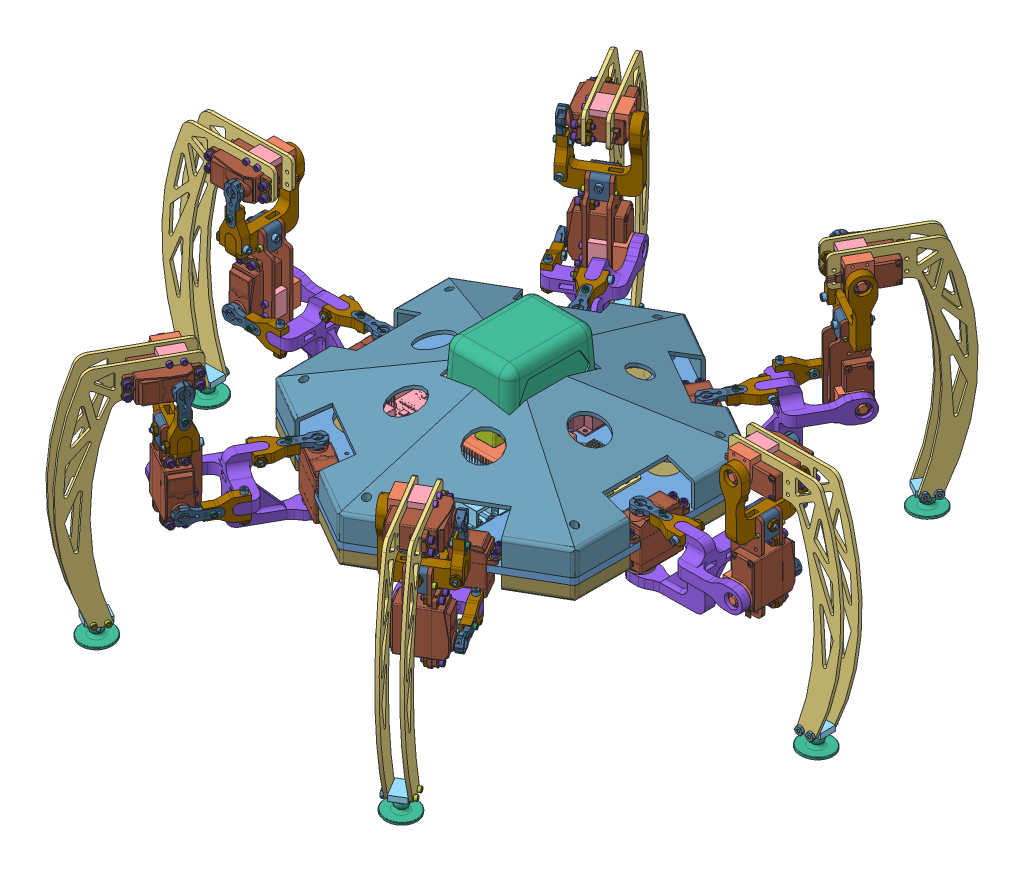
SolidWorks assembly Hexapod_(Hexagonal), configuration Défaut. Lengths in mm.
Overall size (628.94 223.3 579.2).
540 component instances, 32 part files, 38 mates.
Components (placement in the parent):
- Body_(Hexagonal)-1: Body_(Hexagonal) [Défaut] at origin size (278.74 6 320)
- Battery_holder-1: Battery_holder [Default] at (0 14.35 0) x (0 0 1) z (-1 0 0) size (60 19.6 60)
- 12Channel PWM-1: 12Channel PWM [Default] at (77.5 3 0) size (25.4 7.55 66.7)
- 12Channel PWM-2: 12Channel PWM [Default] at (47.4 3 0) size (25.4 7.55 66.7)
- arduinoMega-2: arduinoMega [Detailed] at (-61.35 5 1.27) x (0 0 -1) z (1 0 0) size (108.32 14.5 53.3)
- raspberryPi3B-1: raspberryPi3B [Detailed] at (12.5 5.5 63.95) x (1 0 0) z (0 1 0) size (87.05 58.5 19.5)
- Battery-1: Battery [Défaut] at (0.5853 59.4876 -93.4347) x (-1 0 0) z (0 0 1) size (64.47 74.3 85.78)
  - MAKITA 4.0AH-1: MAKITA 4.0AH [Défaut] at (0.5853 -29.7874 85.4436) size (64.47 57.15 85.78)
  - MAKITA 4.0AH MOBILE-1: MAKITA 4.0AH MOBILE [Défaut] at (0.5853 -39.3124 91.7936) size (45.84 26.68 66.29)
- Foot+Tibia+Femur-1: Foot+Tibia+Femur [Défaut] at (-119.0679 -25 20.1) size (210.19 223.27 63.83) (flexible)
  - Femur-1: Femur [Défaut] at origin size (137.43 61.64 61.08) (flexible)
    - Joint_(Femur_to_tibia)-1: Joint_(Femur_to_tibia) [Défaut] at (-66.4348 29.5 -48.8085) x (0.999924 0 -0.012321) z (0.012321 0 0.999924) size (122 58.8 58.8)
    - Horn_attachment-3: Horn_attachment [Défaut] at (-38.1979 44.8 -29.755) x (0.999924 0 -0.012321) z (0 1 0) size (33 20 8)
    - Horn-3: Horn [Défaut] at (-10.2 48.8 -30.1) x (-0.999924 0 0.012321) z (0 1 0) size (35.39 15.87 6)
    - DS3225MG-3: DS3225MG [Default] at (-10.2 45.8 -30.1) x (0 0 1) z (0 1 0) size (57.25 20.4 45.91)
    - Bearing_mount_(Femur)-1: Bearing_mount_(Femur) [Default] at (2.5 22 -30.1) x (1 0 0) z (0 -1 0) size (35.3 20.2 31)
    - Bearing-3: Bearing [Default] at (-10.2 -6.7498 -30.1) x (0.400474 0 0.916308) z (-0.916308 0 0.400474) size (13.87 4.75 13.87)
    - MSHXNUT 0.112-40-D-N-1: MSHXNUT 0.112-40-D-N [MSHXNUT 0.112-40-D-N] at (-30.1985 40.8 -29.8536) x (-0.510633 0 -0.859799) z (0 1 0) size (6.35 7.33 2.49)
    - HX-SHCS 0.112-40x0.4375x0.4375-N-1: HX-SHCS 0.112-40x0.4375x0.4375-N [HX-SHCS 0.112-40x0.4375x0.4375-N] at (-30.1985 51.6448 -29.8536) x (0 -1 0) z (-0.489292 0 0.87212) size (13.96 4.65 4.65)
    - Narrow FW 0.138-1: Narrow FW 0.138 [Narrow FW 0.138] at (-15.2 31.2 4.7) x (0 -1 0) z (-0.829316 0 -0.55878) size (0.81 7.92 7.92)
    - HX-SHCS 0.138-32x0.5x0.5-N-1: HX-SHCS 0.138-32x0.5x0.5-N [HX-SHCS 0.138-32x0.5x0.5-N] at (-15.2 35.772 4.7) x (0 -1 0) z (0.866025 0 -0.5) size (16.21 5.74 5.74)
    - Narrow FW 0.138-2: Narrow FW 0.138 [Narrow FW 0.138] at (-15.2 31.2 -44.9) x (0 -1 0) z (-0.829316 0 -0.55878) size (0.81 7.92 7.92)
    - Narrow FW 0.138-3: Narrow FW 0.138 [Narrow FW 0.138] at (-5.2 31.2 4.7) x (0 -1 0) z (-0.829316 0 -0.55878) size (0.81 7.92 7.92)
    - Narrow FW 0.138-4: Narrow FW 0.138 [Narrow FW 0.138] at (-5.2 31.2 -44.9) x (0 -1 0) z (-0.829316 0 -0.55878) size (0.81 7.92 7.92)
    - HX-SHCS 0.138-32x0.5x0.5-N-2: HX-SHCS 0.138-32x0.5x0.5-N [HX-SHCS 0.138-32x0.5x0.5-N] at (-15.2 35.772 -44.9) x (0 -1 0) z (0.866025 0 -0.5) size (16.21 5.74 5.74)
    - HX-SHCS 0.138-32x0.5x0.5-N-3: HX-SHCS 0.138-32x0.5x0.5-N [HX-SHCS 0.138-32x0.5x0.5-N] at (-5.2 35.772 4.7) x (0 -1 0) z (0.866025 0 -0.5) size (16.21 5.74 5.74)
    - HX-SHCS 0.138-32x0.5x0.5-N-4: HX-SHCS 0.138-32x0.5x0.5-N [HX-SHCS 0.138-32x0.5x0.5-N] at (-5.2 35.772 -44.9) x (0 -1 0) z (0.866025 0 -0.5) size (16.21 5.74 5.74)
    - MSHXNUT 0.138-32-D-N-1: MSHXNUT 0.138-32-D-N [MSHXNUT 0.138-32-D-N] at (-52.0379 44.8 -16.6879) x (-0.86596 -0.5 0.010671) z (0.012321 0 0.999924) size (7.92 9.15 2.9)
    - HX-SHCS 0.138-32x1x1-N-2: HX-SHCS 0.138-32x1x1-N [HX-SHCS 0.138-32x1x1-N] at (-52.3632 44.8 -43.0867) x (0.012321 0 0.999924) z (-0.86596 -0.5 0.010671) size (28.91 5.74 5.74)
  - Foot_(Long)-4: Foot_(Long) [Défaut] at (-141.7664 117.7478 -37.8795) x (0.999923 0.001668 -0.012321) z (0.012321 0 0.999924) size (104.1 223.13 60.64) (flexible)
    - DS3225MG-1: DS3225MG [Default] at (30.1 10.2 45.8) x (-1 0 0) z (0 0 1) size (57.25 20.4 45.91)
    - Bearing-1: Bearing [Default] at (30.1 10.2 -6.7498) x (-0.568255 0.822853 0) z (0.822853 0.568255 0) size (13.87 4.75 13.87)
    - Bearing_mount_(Foot)-1: Bearing_mount_(Foot) [Default] at (30.1 22.9 8.1) x (0 1 0) z (0 0 -1) size (25.3 20.2 17.1)
    - Foot_(Long)-1: Foot_(Long) [Default] at (18.7 14 25) size (103.08 208 3)
    - Link-1: Link [Default] at (30.1 22.9 11.1) x (0 -1 0) z (0 0 1) size (5 20.2 13.9)
    - Foot_(Long)-2: Foot_(Long) [Default] at (18.7 14 8.1) size (103.08 208 3)
    - Joint_(Foot_to_slipper)-2: Joint_(Foot_to_slipper) [Default] at (-21.9427 -177.5 11.1) x (0 1 0) z (0 0 1) size (15 20.2 13.9)
    - Horn-1: Horn [Défaut] at (30.1 10.2 48.8) x (-0.007987 -0.999968 0) z (0 0 1) size (35.39 15.87 6)
    - Horn_attachment-1: Horn_attachment [Défaut] at (29.8764 -17.7991 44.8) x (0.007987 0.999968 0) z (0 0 1) size (33 20 8)
    - Slipper-1: Slipper [Défaut] at (-21.7184 -191.9896 17.7406) x (0.999392 0.031392 0.015197) z (-0.013787 -0.044657 0.998907) size (30 10.55 30)
    - HX-SHCS 0.112-40x0.4375x0.4375-N-15: HX-SHCS 0.112-40x0.4375x0.4375-N [HX-SHCS 0.112-40x0.4375x0.4375-N] at (29.9403 -9.7994 51.6448) x (0 0 -1) z (0.869991 0.493067 0) size (13.96 4.65 4.65)
    - MSHXNUT 0.112-40-D-N-7: MSHXNUT 0.112-40-D-N [MSHXNUT 0.112-40-D-N] at (29.9403 -9.7994 40.8) x (-0.007987 -0.999968 0) z (0 0 1) size (6.35 7.33 2.49)
    - HX-SHCS 0.112-40x0.875x0.875-N-9: HX-SHCS 0.112-40x0.875x0.875-N [HX-SHCS 0.112-40x0.875x0.875-N] at (-26.9427 -177.5 30.8448) x (0 0 -1) z (0 1 0) size (25.07 4.65 4.65)
    - MSHXNUT 0.112-40-D-N-4: MSHXNUT 0.112-40-D-N [MSHXNUT 0.112-40-D-N] at (-26.9427 -177.5 8.1) x (0.866025 -0.5 0) z (0 0 1) size (6.35 7.33 2.49)
    - HX-SHCS 0.112-40x0.875x0.875-N-11: HX-SHCS 0.112-40x0.875x0.875-N [HX-SHCS 0.112-40x0.875x0.875-N] at (-16.9427 -177.5 30.8448) x (0 0 -1) z (0 1 0) size (25.07 4.65 4.65)
    - MSHXNUT 0.112-40-D-N-6: MSHXNUT 0.112-40-D-N [MSHXNUT 0.112-40-D-N] at (-16.9427 -177.5 8.1) x (0.866025 -0.5 0) z (0 0 1) size (6.35 7.33 2.49)
    - HX-SHCS 0.112-40x1x0.75-N-13: HX-SHCS 0.112-40x1x0.75-N [HX-SHCS 0.112-40x1x0.75-N] at (25.1 22.9 30.8448) x (0 0 -1) z (0 1 0) size (28.24 4.65 4.65)
    - HX-SHCS 0.112-40x1x0.75-N-14: HX-SHCS 0.112-40x1x0.75-N [HX-SHCS 0.112-40x1x0.75-N] at (35.1 22.9 30.8448) x (0 0 -1) z (0 1 0) size (28.24 4.65 4.65)
    - HX-SHCS 0.138-32x0.5x0.5-N-14: HX-SHCS 0.138-32x0.5x0.5-N [HX-SHCS 0.138-32x0.5x0.5-N] at (-4.7 5.2 35.772) x (0 0 -1) z (0.866025 0.5 0) size (16.21 5.74 5.74)
    - Narrow FW 0.138-1: Narrow FW 0.138 [Narrow FW 0.138] at (-4.7 5.2 31.2) x (0 0 -1) z (-0.829316 0.55878 0) size (0.81 7.92 7.92)
    - MSHXNUT 0.138-32-D-N-1: MSHXNUT 0.138-32-D-N [MSHXNUT 0.138-32-D-N] at (-4.7 5.2 25) x (0.866025 0.5 0) z (0 0 1) size (7.92 9.15 2.9)
    - MSHXNUT 0.138-32-D-N-2: MSHXNUT 0.138-32-D-N [MSHXNUT 0.138-32-D-N] at (44.9 5.2 25) x (0.866025 0.5 0) z (0 0 1) size (7.92 9.15 2.9)
    - MSHXNUT 0.138-32-D-N-3: MSHXNUT 0.138-32-D-N [MSHXNUT 0.138-32-D-N] at (-4.7 15.2 25) x (0.866025 0.5 0) z (0 0 1) size (7.92 9.15 2.9)
    - MSHXNUT 0.138-32-D-N-4: MSHXNUT 0.138-32-D-N [MSHXNUT 0.138-32-D-N] at (44.9 15.2 25) x (0.866025 0.5 0) z (0 0 1) size (7.92 9.15 2.9)
    - HX-SHCS 0.138-32x0.5x0.5-N-15: HX-SHCS 0.138-32x0.5x0.5-N [HX-SHCS 0.138-32x0.5x0.5-N] at (44.9 5.2 35.772) x (0 0 -1) z (0.866025 0.5 0) size (16.21 5.74 5.74)
    - HX-SHCS 0.138-32x0.5x0.5-N-16: HX-SHCS 0.138-32x0.5x0.5-N [HX-SHCS 0.138-32x0.5x0.5-N] at (-4.7 15.2 35.772) x (0 0 -1) z (0.866025 0.5 0) size (16.21 5.74 5.74)
    - HX-SHCS 0.138-32x0.5x0.5-N-17: HX-SHCS 0.138-32x0.5x0.5-N [HX-SHCS 0.138-32x0.5x0.5-N] at (44.9 15.2 35.772) x (0 0 -1) z (0.866025 0.5 0) size (16.21 5.74 5.74)
    - Narrow FW 0.138-2: Narrow FW 0.138 [Narrow FW 0.138] at (44.9 5.2 31.2) x (0 0 -1) z (-0.829316 0.55878 0) size (0.81 7.92 7.92)
    - Narrow FW 0.138-3: Narrow FW 0.138 [Narrow FW 0.138] at (-4.7 15.2 31.2) x (0 0 -1) z (-0.829316 0.55878 0) size (0.81 7.92 7.92)
    - Narrow FW 0.138-4: Narrow FW 0.138 [Narrow FW 0.138] at (44.9 15.2 31.2) x (0 0 -1) z (-0.829316 0.55878 0) size (0.81 7.92 7.92)
  - Tibia-3: Tibia [Défaut] at (-122.5709 19.4647 -38.1161) x (-0.006318 -0.99998 0.000078) z (0.012321 0 0.999924) size (129.02 61.26 61.64) (flexible)
    - Joint_(Tibia_to_foot)-1: Joint_(Tibia_to_foot) [Défaut] at (-62.6 10.2 -10) size (64 20 58.8)
    - DS3225MG-2: DS3225MG [Default] at (-10.1 10.2 45.8) x (-1 0 0) z (0 0 1) size (57.25 20.4 45.91)
    - Link-3: Link [Default] at (-10.1 22.9 11.1) x (0 -1 0) z (0 0 1) size (5 20.2 13.9)
    - Horn-2: Horn [Défaut] at (-10.1 10.2 48.8) x (-0.006319 0.99998 0) z (0 0 1) size (35.39 15.87 6)
    - Horn_attachment-2: Horn_attachment [Défaut] at (-10.2769 38.1994 44.8) x (0.006319 -0.99998 0) z (0 0 1) size (33 20 8)
    - Joint_attachment_(Tibia)-1: Joint_attachment_(Tibia) [Défaut] at (-62.6 10.2 25) size (19 20.4 13.9)
    - Tibia-1: Tibia [Défaut] at (-62.6 10.2 28) size (80 28 3)
    - Tibia-2: Tibia [Défaut] at (-62.6 10.2 11.1) size (80 28 3)
    - Bearing_mount_(Foot)-2: Bearing_mount_(Foot) [Default] at (-10.1 22.9 8.1) x (0 1 0) z (0 0 -1) size (25.3 20.2 17.1)
    - Bearing-2: Bearing [Default] at (-10.1 10.2 -6.7498) x (-0.993915 0.110147 0) z (0.110147 0.993915 0) size (13.87 4.75 13.87)
    - HX-SHCS 0.112-40x0.4375x0.4375-N-1: HX-SHCS 0.112-40x0.4375x0.4375-N [HX-SHCS 0.112-40x0.4375x0.4375-N] at (-10.2264 30.1996 51.6448) x (0 0 -1) z (-0.862849 -0.505462 0) size (13.96 4.65 4.65)
    - MSHXNUT 0.112-40-D-N-1: MSHXNUT 0.112-40-D-N [MSHXNUT 0.112-40-D-N] at (-10.2264 30.1996 40.8) x (-0.006319 0.99998 0) z (0 0 1) size (6.35 7.33 2.49)
    - HX-SHCS 0.112-40x1x0.75-N-1: HX-SHCS 0.112-40x1x0.75-N [HX-SHCS 0.112-40x1x0.75-N] at (-15.1 22.9 30.8448) x (0 0 -1) z (0 1 0) size (28.24 4.65 4.65)
    - HX-SHCS 0.112-40x1x0.75-N-2: HX-SHCS 0.112-40x1x0.75-N [HX-SHCS 0.112-40x1x0.75-N] at (-5.1 22.9 30.8448) x (0 0 -1) z (0 1 0) size (28.24 4.65 4.65)
    - HX-SHCS 0.138-32x0.5x0.5-N-1: HX-SHCS 0.138-32x0.5x0.5-N [HX-SHCS 0.138-32x0.5x0.5-N] at (-44.9 5.2 35.772) x (0 0 -1) z (0.866025 0.5 0) size (16.21 5.74 5.74)
    - Narrow FW 0.138-1: Narrow FW 0.138 [Narrow FW 0.138] at (-44.9 5.2 31.2) x (0 0 -1) z (-0.54947 -0.835514 0) size (0.81 7.92 7.92)
    - MSHXNUT 0.138-32-D-N-1: MSHXNUT 0.138-32-D-N [MSHXNUT 0.138-32-D-N] at (-44.9 5.2 25) x (0.866025 0.5 0) z (0 0 1) size (7.92 9.15 2.9)
    - MSHXNUT 0.138-32-D-N-2: MSHXNUT 0.138-32-D-N [MSHXNUT 0.138-32-D-N] at (4.7 5.2 25) x (0.866025 0.5 0) z (0 0 1) size (7.92 9.15 2.9)
    - MSHXNUT 0.138-32-D-N-3: MSHXNUT 0.138-32-D-N [MSHXNUT 0.138-32-D-N] at (-44.9 15.2 25) x (0.866025 0.5 0) z (0 0 1) size (7.92 9.15 2.9)
    - MSHXNUT 0.138-32-D-N-4: MSHXNUT 0.138-32-D-N [MSHXNUT 0.138-32-D-N] at (4.7 15.2 25) x (0.866025 0.5 0) z (0 0 1) size (7.92 9.15 2.9)
    - Narrow FW 0.138-2: Narrow FW 0.138 [Narrow FW 0.138] at (4.7 5.2 31.2) x (0 0 -1) z (-0.54947 -0.835514 0) size (0.81 7.92 7.92)
    - Narrow FW 0.138-3: Narrow FW 0.138 [Narrow FW 0.138] at (-44.9 15.2 31.2) x (0 0 -1) z (-0.54947 -0.835514 0) size (0.81 7.92 7.92)
    - Narrow FW 0.138-4: Narrow FW 0.138 [Narrow FW 0.138] at (4.7 15.2 31.2) x (0 0 -1) z (-0.54947 -0.835514 0) size (0.81 7.92 7.92)
    - HX-SHCS 0.138-32x0.5x0.5-N-2: HX-SHCS 0.138-32x0.5x0.5-N [HX-SHCS 0.138-32x0.5x0.5-N] at (4.7 5.2 35.772) x (0 0 -1) z (0.866025 0.5 0) size (16.21 5.74 5.74)
    - HX-SHCS 0.138-32x0.5x0.5-N-3: HX-SHCS 0.138-32x0.5x0.5-N [HX-SHCS 0.138-32x0.5x0.5-N] at (-44.9 15.2 35.772) x (0 0 -1) z (0.866025 0.5 0) size (16.21 5.74 5.74)
    - HX-SHCS 0.138-32x0.5x0.5-N-4: HX-SHCS 0.138-32x0.5x0.5-N [HX-SHCS 0.138-32x0.5x0.5-N] at (4.7 15.2 35.772) x (0 0 -1) z (0.866025 0.5 0) size (16.21 5.74 5.74)
    - HX-SHCS 0.112-40x0.875x0.875-N-1: HX-SHCS 0.112-40x0.875x0.875-N [HX-SHCS 0.112-40x0.875x0.875-N] at (-57.6 17.8 30.8448) x (0 0 -1) z (0 1 0) size (25.07 4.65 4.65)
    - HX-SHCS 0.112-40x0.875x0.875-N-2: HX-SHCS 0.112-40x0.875x0.875-N [HX-SHCS 0.112-40x0.875x0.875-N] at (-57.6 2.6 30.8448) x (0 0 -1) z (0 1 0) size (25.07 4.65 4.65)
    - HX-SHCS 0.138-32x1x1-N-1: HX-SHCS 0.138-32x1x1-N [HX-SHCS 0.138-32x1x1-N] at (-62.6 23.9052 18.05) x (0 -1 0) z (1 0 0) size (28.91 5.74 5.74)
    - MSHXNUT 0.138-32-D-N-5: MSHXNUT 0.138-32-D-N [MSHXNUT 0.138-32-D-N] at (-62.6 -2.8956 18.05) x (1 0 0) z (0 -1 0) size (7.92 9.15 2.9)
  - HX-SHCS 0.138-32x1x1-N-1: HX-SHCS 0.138-32x1x1-N [HX-SHCS 0.138-32x1x1-N] at (-69.7593 43.0052 6.0366) x (0 -1 0) z (-0.87212 0 -0.489292) size (28.91 5.74 5.74)
  - MSHXNUT 0.138-32-D-N-1: MSHXNUT 0.138-32-D-N [MSHXNUT 0.138-32-D-N] at (-69.7593 16.6044 6.0366) x (-0.87212 0 -0.489292) z (0 -1 0) size (7.92 9.15 2.9)
  - MSHXNUT 0.138-32-D-N-2: MSHXNUT 0.138-32-D-N [MSHXNUT 0.138-32-D-N] at (-124.2935 86.0804 6.7086) x (-0.000689 0.866008 -0.500029) z (-0.999904 0.006319 0.012321) size (7.92 9.15 2.9)
  - HX-SHCS 0.138-32x1x1-N-2: HX-SHCS 0.138-32x1x1-N [HX-SHCS 0.138-32x1x1-N] at (-97.8952 85.9135 6.3833) x (-0.999904 0.006319 0.012321) z (-0.012321 0 -0.999924) size (28.91 5.74 5.74)
- Foot+Tibia+Femur-7: Foot+Tibia+Femur [Défaut] at (-42.1268 -25 113.1658) x (0.5 0 -0.866025) z (0.866025 0 0.5) size (210.19 223.27 63.83) (flexible)
  - Femur-1: Femur [Défaut] at origin size (137.43 61.64 61.08) (flexible)
    - Joint_(Femur_to_tibia)-1: Joint_(Femur_to_tibia) [Défaut] at (-66.4348 29.5 -48.8085) x (0.999924 0 -0.012321) z (0.012321 0 0.999924) size (122 58.8 58.8)
    - Horn_attachment-3: Horn_attachment [Défaut] at (-38.1979 44.8 -29.755) x (0.999924 0 -0.012321) z (0 1 0) size (33 20 8)
    - Horn-3: Horn [Défaut] at (-10.2 48.8 -30.1) x (-0.999924 0 0.012321) z (0 1 0) size (35.39 15.87 6)
    - DS3225MG-3: DS3225MG [Default] at (-10.2 45.8 -30.1) x (0 0 1) z (0 1 0) size (57.25 20.4 45.91)
    - Bearing_mount_(Femur)-1: Bearing_mount_(Femur) [Default] at (2.5 22 -30.1) x (1 0 0) z (0 -1 0) size (35.3 20.2 31)
    - Bearing-3: Bearing [Default] at (-10.2 -6.7498 -30.1) x (0.400474 0 0.916308) z (-0.916308 0 0.400474) size (13.87 4.75 13.87)
    - MSHXNUT 0.112-40-D-N-1: MSHXNUT 0.112-40-D-N [MSHXNUT 0.112-40-D-N] at (-30.1985 40.8 -29.8536) x (-0.510633 0 -0.859799) z (0 1 0) size (6.35 7.33 2.49)
    - HX-SHCS 0.112-40x0.4375x0.4375-N-1: HX-SHCS 0.112-40x0.4375x0.4375-N [HX-SHCS 0.112-40x0.4375x0.4375-N] at (-30.1985 51.6448 -29.8536) x (0 -1 0) z (-0.489292 0 0.87212) size (13.96 4.65 4.65)
    - Narrow FW 0.138-1: Narrow FW 0.138 [Narrow FW 0.138] at (-15.2 31.2 4.7) x (0 -1 0) z (-0.829316 0 -0.55878) size (0.81 7.92 7.92)
    - HX-SHCS 0.138-32x0.5x0.5-N-1: HX-SHCS 0.138-32x0.5x0.5-N [HX-SHCS 0.138-32x0.5x0.5-N] at (-15.2 35.772 4.7) x (0 -1 0) z (0.866025 0 -0.5) size (16.21 5.74 5.74)
    - Narrow FW 0.138-2: Narrow FW 0.138 [Narrow FW 0.138] at (-15.2 31.2 -44.9) x (0 -1 0) z (-0.829316 0 -0.55878) size (0.81 7.92 7.92)
    - Narrow FW 0.138-3: Narrow FW 0.138 [Narrow FW 0.138] at (-5.2 31.2 4.7) x (0 -1 0) z (-0.829316 0 -0.55878) size (0.81 7.92 7.92)
    - Narrow FW 0.138-4: Narrow FW 0.138 [Narrow FW 0.138] at (-5.2 31.2 -44.9) x (0 -1 0) z (-0.829316 0 -0.55878) size (0.81 7.92 7.92)
    - HX-SHCS 0.138-32x0.5x0.5-N-2: HX-SHCS 0.138-32x0.5x0.5-N [HX-SHCS 0.138-32x0.5x0.5-N] at (-15.2 35.772 -44.9) x (0 -1 0) z (0.866025 0 -0.5) size (16.21 5.74 5.74)
    - HX-SHCS 0.138-32x0.5x0.5-N-3: HX-SHCS 0.138-32x0.5x0.5-N [HX-SHCS 0.138-32x0.5x0.5-N] at (-5.2 35.772 4.7) x (0 -1 0) z (0.866025 0 -0.5) size (16.21 5.74 5.74)
    - HX-SHCS 0.138-32x0.5x0.5-N-4: HX-SHCS 0.138-32x0.5x0.5-N [HX-SHCS 0.138-32x0.5x0.5-N] at (-5.2 35.772 -44.9) x (0 -1 0) z (0.866025 0 -0.5) size (16.21 5.74 5.74)
    - MSHXNUT 0.138-32-D-N-1: MSHXNUT 0.138-32-D-N [MSHXNUT 0.138-32-D-N] at (-52.0379 44.8 -16.6879) x (-0.86596 -0.5 0.010671) z (0.012321 0 0.999924) size (7.92 9.15 2.9)
    - HX-SHCS 0.138-32x1x1-N-2: HX-SHCS 0.138-32x1x1-N [HX-SHCS 0.138-32x1x1-N] at (-52.3632 44.8 -43.0867) x (0.012321 0 0.999924) z (-0.86596 -0.5 0.010671) size (28.91 5.74 5.74)
  - Foot_(Long)-4: Foot_(Long) [Défaut] at (-141.7664 117.7478 -37.8795) x (0.999923 0.001668 -0.012321) z (0.012321 0 0.999924) size (104.1 223.13 60.64) (flexible)
    - DS3225MG-1: DS3225MG [Default] at (30.1 10.2 45.8) x (-1 0 0) z (0 0 1) size (57.25 20.4 45.91)
    - Bearing-1: Bearing [Default] at (30.1 10.2 -6.7498) x (-0.568255 0.822853 0) z (0.822853 0.568255 0) size (13.87 4.75 13.87)
    - Bearing_mount_(Foot)-1: Bearing_mount_(Foot) [Default] at (30.1 22.9 8.1) x (0 1 0) z (0 0 -1) size (25.3 20.2 17.1)
    - Foot_(Long)-1: Foot_(Long) [Default] at (18.7 14 25) size (103.08 208 3)
    - Link-1: Link [Default] at (30.1 22.9 11.1) x (0 -1 0) z (0 0 1) size (5 20.2 13.9)
    - Foot_(Long)-2: Foot_(Long) [Default] at (18.7 14 8.1) size (103.08 208 3)
    - Joint_(Foot_to_slipper)-2: Joint_(Foot_to_slipper) [Default] at (-21.9427 -177.5 11.1) x (0 1 0) z (0 0 1) size (15 20.2 13.9)
    - Horn-1: Horn [Défaut] at (30.1 10.2 48.8) x (-0.007987 -0.999968 0) z (0 0 1) size (35.39 15.87 6)
    - Horn_attachment-1: Horn_attachment [Défaut] at (29.8764 -17.7991 44.8) x (0.007987 0.999968 0) z (0 0 1) size (33 20 8)
    - Slipper-1: Slipper [Défaut] at (-21.7184 -191.9896 17.7406) x (0.999392 0.031392 0.015197) z (-0.013787 -0.044657 0.998907) size (30 10.55 30)
    - HX-SHCS 0.112-40x0.4375x0.4375-N-15: HX-SHCS 0.112-40x0.4375x0.4375-N [HX-SHCS 0.112-40x0.4375x0.4375-N] at (29.9403 -9.7994 51.6448) x (0 0 -1) z (0.869991 0.493067 0) size (13.96 4.65 4.65)
    - MSHXNUT 0.112-40-D-N-7: MSHXNUT 0.112-40-D-N [MSHXNUT 0.112-40-D-N] at (29.9403 -9.7994 40.8) x (-0.007987 -0.999968 0) z (0 0 1) size (6.35 7.33 2.49)
    - HX-SHCS 0.112-40x0.875x0.875-N-9: HX-SHCS 0.112-40x0.875x0.875-N [HX-SHCS 0.112-40x0.875x0.875-N] at (-26.9427 -177.5 30.8448) x (0 0 -1) z (0 1 0) size (25.07 4.65 4.65)
    - MSHXNUT 0.112-40-D-N-4: MSHXNUT 0.112-40-D-N [MSHXNUT 0.112-40-D-N] at (-26.9427 -177.5 8.1) x (0.866025 -0.5 0) z (0 0 1) size (6.35 7.33 2.49)
    - HX-SHCS 0.112-40x0.875x0.875-N-11: HX-SHCS 0.112-40x0.875x0.875-N [HX-SHCS 0.112-40x0.875x0.875-N] at (-16.9427 -177.5 30.8448) x (0 0 -1) z (0 1 0) size (25.07 4.65 4.65)
    - MSHXNUT 0.112-40-D-N-6: MSHXNUT 0.112-40-D-N [MSHXNUT 0.112-40-D-N] at (-16.9427 -177.5 8.1) x (0.866025 -0.5 0) z (0 0 1) size (6.35 7.33 2.49)
    - HX-SHCS 0.112-40x1x0.75-N-13: HX-SHCS 0.112-40x1x0.75-N [HX-SHCS 0.112-40x1x0.75-N] at (25.1 22.9 30.8448) x (0 0 -1) z (0 1 0) size (28.24 4.65 4.65)
    - HX-SHCS 0.112-40x1x0.75-N-14: HX-SHCS 0.112-40x1x0.75-N [HX-SHCS 0.112-40x1x0.75-N] at (35.1 22.9 30.8448) x (0 0 -1) z (0 1 0) size (28.24 4.65 4.65)
    - HX-SHCS 0.138-32x0.5x0.5-N-14: HX-SHCS 0.138-32x0.5x0.5-N [HX-SHCS 0.138-32x0.5x0.5-N] at (-4.7 5.2 35.772) x (0 0 -1) z (0.866025 0.5 0) size (16.21 5.74 5.74)
    - Narrow FW 0.138-1: Narrow FW 0.138 [Narrow FW 0.138] at (-4.7 5.2 31.2) x (0 0 -1) z (-0.829316 0.55878 0) size (0.81 7.92 7.92)
    - MSHXNUT 0.138-32-D-N-1: MSHXNUT 0.138-32-D-N [MSHXNUT 0.138-32-D-N] at (-4.7 5.2 25) x (0.866025 0.5 0) z (0 0 1) size (7.92 9.15 2.9)
    - MSHXNUT 0.138-32-D-N-2: MSHXNUT 0.138-32-D-N [MSHXNUT 0.138-32-D-N] at (44.9 5.2 25) x (0.866025 0.5 0) z (0 0 1) size (7.92 9.15 2.9)
    - MSHXNUT 0.138-32-D-N-3: MSHXNUT 0.138-32-D-N [MSHXNUT 0.138-32-D-N] at (-4.7 15.2 25) x (0.866025 0.5 0) z (0 0 1) size (7.92 9.15 2.9)
    - MSHXNUT 0.138-32-D-N-4: MSHXNUT 0.138-32-D-N [MSHXNUT 0.138-32-D-N] at (44.9 15.2 25) x (0.866025 0.5 0) z (0 0 1) size (7.92 9.15 2.9)
    - HX-SHCS 0.138-32x0.5x0.5-N-15: HX-SHCS 0.138-32x0.5x0.5-N [HX-SHCS 0.138-32x0.5x0.5-N] at (44.9 5.2 35.772) x (0 0 -1) z (0.866025 0.5 0) size (16.21 5.74 5.74)
    - HX-SHCS 0.138-32x0.5x0.5-N-16: HX-SHCS 0.138-32x0.5x0.5-N [HX-SHCS 0.138-32x0.5x0.5-N] at (-4.7 15.2 35.772) x (0 0 -1) z (0.866025 0.5 0) size (16.21 5.74 5.74)
    - HX-SHCS 0.138-32x0.5x0.5-N-17: HX-SHCS 0.138-32x0.5x0.5-N [HX-SHCS 0.138-32x0.5x0.5-N] at (44.9 15.2 35.772) x (0 0 -1) z (0.866025 0.5 0) size (16.21 5.74 5.74)
    - Narrow FW 0.138-2: Narrow FW 0.138 [Narrow FW 0.138] at (44.9 5.2 31.2) x (0 0 -1) z (-0.829316 0.55878 0) size (0.81 7.92 7.92)
    - Narrow FW 0.138-3: Narrow FW 0.138 [Narrow FW 0.138] at (-4.7 15.2 31.2) x (0 0 -1) z (-0.829316 0.55878 0) size (0.81 7.92 7.92)
    - Narrow FW 0.138-4: Narrow FW 0.138 [Narrow FW 0.138] at (44.9 15.2 31.2) x (0 0 -1) z (-0.829316 0.55878 0) size (0.81 7.92 7.92)
  - Tibia-3: Tibia [Défaut] at (-122.5709 19.4647 -38.1161) x (-0.006318 -0.99998 0.000078) z (0.012321 0 0.999924) size (129.02 61.26 61.64) (flexible)
    - Joint_(Tibia_to_foot)-1: Joint_(Tibia_to_foot) [Défaut] at (-62.6 10.2 -10) size (64 20 58.8)
    - DS3225MG-2: DS3225MG [Default] at (-10.1 10.2 45.8) x (-1 0 0) z (0 0 1) size (57.25 20.4 45.91)
    - Link-3: Link [Default] at (-10.1 22.9 11.1) x (0 -1 0) z (0 0 1) size (5 20.2 13.9)
    - Horn-2: Horn [Défaut] at (-10.1 10.2 48.8) x (-0.006319 0.99998 0) z (0 0 1) size (35.39 15.87 6)
    - Horn_attachment-2: Horn_attachment [Défaut] at (-10.2769 38.1994 44.8) x (0.006319 -0.99998 0) z (0 0 1) size (33 20 8)
    - Joint_attachment_(Tibia)-1: Joint_attachment_(Tibia) [Défaut] at (-62.6 10.2 25) size (19 20.4 13.9)
    - Tibia-1: Tibia [Défaut] at (-62.6 10.2 28) size (80 28 3)
    - Tibia-2: Tibia [Défaut] at (-62.6 10.2 11.1) size (80 28 3)
    - Bearing_mount_(Foot)-2: Bearing_mount_(Foot) [Default] at (-10.1 22.9 8.1) x (0 1 0) z (0 0 -1) size (25.3 20.2 17.1)
    - Bearing-2: Bearing [Default] at (-10.1 10.2 -6.7498) x (-0.993915 0.110147 0) z (0.110147 0.993915 0) size (13.87 4.75 13.87)
    - HX-SHCS 0.112-40x0.4375x0.4375-N-1: HX-SHCS 0.112-40x0.4375x0.4375-N [HX-SHCS 0.112-40x0.4375x0.4375-N] at (-10.2264 30.1996 51.6448) x (0 0 -1) z (-0.862849 -0.505462 0) size (13.96 4.65 4.65)
    - MSHXNUT 0.112-40-D-N-1: MSHXNUT 0.112-40-D-N [MSHXNUT 0.112-40-D-N] at (-10.2264 30.1996 40.8) x (-0.006319 0.99998 0) z (0 0 1) size (6.35 7.33 2.49)
    - HX-SHCS 0.112-40x1x0.75-N-1: HX-SHCS 0.112-40x1x0.75-N [HX-SHCS 0.112-40x1x0.75-N] at (-15.1 22.9 30.8448) x (0 0 -1) z (0 1 0) size (28.24 4.65 4.65)
    - HX-SHCS 0.112-40x1x0.75-N-2: HX-SHCS 0.112-40x1x0.75-N [HX-SHCS 0.112-40x1x0.75-N] at (-5.1 22.9 30.8448) x (0 0 -1) z (0 1 0) size (28.24 4.65 4.65)
    - HX-SHCS 0.138-32x0.5x0.5-N-1: HX-SHCS 0.138-32x0.5x0.5-N [HX-SHCS 0.138-32x0.5x0.5-N] at (-44.9 5.2 35.772) x (0 0 -1) z (0.866025 0.5 0) size (16.21 5.74 5.74)
    - Narrow FW 0.138-1: Narrow FW 0.138 [Narrow FW 0.138] at (-44.9 5.2 31.2) x (0 0 -1) z (-0.54947 -0.835514 0) size (0.81 7.92 7.92)
    - MSHXNUT 0.138-32-D-N-1: MSHXNUT 0.138-32-D-N [MSHXNUT 0.138-32-D-N] at (-44.9 5.2 25) x (0.866025 0.5 0) z (0 0 1) size (7.92 9.15 2.9)
    - MSHXNUT 0.138-32-D-N-2: MSHXNUT 0.138-32-D-N [MSHXNUT 0.138-32-D-N] at (4.7 5.2 25) x (0.866025 0.5 0) z (0 0 1) size (7.92 9.15 2.9)
    - MSHXNUT 0.138-32-D-N-3: MSHXNUT 0.138-32-D-N [MSHXNUT 0.138-32-D-N] at (-44.9 15.2 25) x (0.866025 0.5 0) z (0 0 1) size (7.92 9.15 2.9)
    - MSHXNUT 0.138-32-D-N-4: MSHXNUT 0.138-32-D-N [MSHXNUT 0.138-32-D-N] at (4.7 15.2 25) x (0.866025 0.5 0) z (0 0 1) size (7.92 9.15 2.9)
    - Narrow FW 0.138-2: Narrow FW 0.138 [Narrow FW 0.138] at (4.7 5.2 31.2) x (0 0 -1) z (-0.54947 -0.835514 0) size (0.81 7.92 7.92)
    - Narrow FW 0.138-3: Narrow FW 0.138 [Narrow FW 0.138] at (-44.9 15.2 31.2) x (0 0 -1) z (-0.54947 -0.835514 0) size (0.81 7.92 7.92)
    - Narrow FW 0.138-4: Narrow FW 0.138 [Narrow FW 0.138] at (4.7 15.2 31.2) x (0 0 -1) z (-0.54947 -0.835514 0) size (0.81 7.92 7.92)
    - HX-SHCS 0.138-32x0.5x0.5-N-2: HX-SHCS 0.138-32x0.5x0.5-N [HX-SHCS 0.138-32x0.5x0.5-N] at (4.7 5.2 35.772) x (0 0 -1) z (0.866025 0.5 0) size (16.21 5.74 5.74)
    - HX-SHCS 0.138-32x0.5x0.5-N-3: HX-SHCS 0.138-32x0.5x0.5-N [HX-SHCS 0.138-32x0.5x0.5-N] at (-44.9 15.2 35.772) x (0 0 -1) z (0.866025 0.5 0) size (16.21 5.74 5.74)
    - HX-SHCS 0.138-32x0.5x0.5-N-4: HX-SHCS 0.138-32x0.5x0.5-N [HX-SHCS 0.138-32x0.5x0.5-N] at (4.7 15.2 35.772) x (0 0 -1) z (0.866025 0.5 0) size (16.21 5.74 5.74)
    - HX-SHCS 0.112-40x0.875x0.875-N-1: HX-SHCS 0.112-40x0.875x0.875-N [HX-SHCS 0.112-40x0.875x0.875-N] at (-57.6 17.8 30.8448) x (0 0 -1) z (0 1 0) size (25.07 4.65 4.65)
    - HX-SHCS 0.112-40x0.875x0.875-N-2: HX-SHCS 0.112-40x0.875x0.875-N [HX-SHCS 0.112-40x0.875x0.875-N] at (-57.6 2.6 30.8448) x (0 0 -1) z (0 1 0) size (25.07 4.65 4.65)
    - HX-SHCS 0.138-32x1x1-N-1: HX-SHCS 0.138-32x1x1-N [HX-SHCS 0.138-32x1x1-N] at (-62.6 23.9052 18.05) x (0 -1 0) z (1 0 0) size (28.91 5.74 5.74)
    - MSHXNUT 0.138-32-D-N-5: MSHXNUT 0.138-32-D-N [MSHXNUT 0.138-32-D-N] at (-62.6 -2.8956 18.05) x (1 0 0) z (0 -1 0) size (7.92 9.15 2.9)
  - HX-SHCS 0.138-32x1x1-N-1: HX-SHCS 0.138-32x1x1-N [HX-SHCS 0.138-32x1x1-N] at (-69.7593 43.0052 6.0366) x (0 -1 0) z (-0.87212 0 -0.489292) size (28.91 5.74 5.74)
  - MSHXNUT 0.138-32-D-N-1: MSHXNUT 0.138-32-D-N [MSHXNUT 0.138-32-D-N] at (-69.7593 16.6044 6.0366) x (-0.87212 0 -0.489292) z (0 -1 0) size (7.92 9.15 2.9)
  - MSHXNUT 0.138-32-D-N-2: MSHXNUT 0.138-32-D-N [MSHXNUT 0.138-32-D-N] at (-124.2935 86.0804 6.7086) x (-0.000689 0.866008 -0.500029) z (-0.999904 0.006319 0.012321) size (7.92 9.15 2.9)
  - HX-SHCS 0.138-32x1x1-N-2: HX-SHCS 0.138-32x1x1-N [HX-SHCS 0.138-32x1x1-N] at (-97.8952 85.9135 6.3833) x (-0.999904 0.006319 0.012321) z (-0.012321 0 -0.999924) size (28.91 5.74 5.74)
- Foot+Tibia+Femur-8: Foot+Tibia+Femur [Défaut] at (76.9411 -25 93.0658) x (-0.5 0 -0.866025) z (0.866025 0 -0.5) size (210.19 223.27 63.83) (flexible)
  - Femur-1: Femur [Défaut] at origin size (137.43 61.64 61.08) (flexible)
    - Joint_(Femur_to_tibia)-1: Joint_(Femur_to_tibia) [Défaut] at (-66.4348 29.5 -48.8085) x (0.999924 0 -0.012321) z (0.012321 0 0.999924) size (122 58.8 58.8)
    - Horn_attachment-3: Horn_attachment [Défaut] at (-38.1979 44.8 -29.755) x (0.999924 0 -0.012321) z (0 1 0) size (33 20 8)
    - Horn-3: Horn [Défaut] at (-10.2 48.8 -30.1) x (-0.999924 0 0.012321) z (0 1 0) size (35.39 15.87 6)
    - DS3225MG-3: DS3225MG [Default] at (-10.2 45.8 -30.1) x (0 0 1) z (0 1 0) size (57.25 20.4 45.91)
    - Bearing_mount_(Femur)-1: Bearing_mount_(Femur) [Default] at (2.5 22 -30.1) x (1 0 0) z (0 -1 0) size (35.3 20.2 31)
    - Bearing-3: Bearing [Default] at (-10.2 -6.7498 -30.1) x (0.400474 0 0.916308) z (-0.916308 0 0.400474) size (13.87 4.75 13.87)
    - MSHXNUT 0.112-40-D-N-1: MSHXNUT 0.112-40-D-N [MSHXNUT 0.112-40-D-N] at (-30.1985 40.8 -29.8536) x (-0.510633 0 -0.859799) z (0 1 0) size (6.35 7.33 2.49)
    - HX-SHCS 0.112-40x0.4375x0.4375-N-1: HX-SHCS 0.112-40x0.4375x0.4375-N [HX-SHCS 0.112-40x0.4375x0.4375-N] at (-30.1985 51.6448 -29.8536) x (0 -1 0) z (-0.489292 0 0.87212) size (13.96 4.65 4.65)
    - Narrow FW 0.138-1: Narrow FW 0.138 [Narrow FW 0.138] at (-15.2 31.2 4.7) x (0 -1 0) z (-0.829316 0 -0.55878) size (0.81 7.92 7.92)
    - HX-SHCS 0.138-32x0.5x0.5-N-1: HX-SHCS 0.138-32x0.5x0.5-N [HX-SHCS 0.138-32x0.5x0.5-N] at (-15.2 35.772 4.7) x (0 -1 0) z (0.866025 0 -0.5) size (16.21 5.74 5.74)
    - Narrow FW 0.138-2: Narrow FW 0.138 [Narrow FW 0.138] at (-15.2 31.2 -44.9) x (0 -1 0) z (-0.829316 0 -0.55878) size (0.81 7.92 7.92)
    - Narrow FW 0.138-3: Narrow FW 0.138 [Narrow FW 0.138] at (-5.2 31.2 4.7) x (0 -1 0) z (-0.829316 0 -0.55878) size (0.81 7.92 7.92)
    - Narrow FW 0.138-4: Narrow FW 0.138 [Narrow FW 0.138] at (-5.2 31.2 -44.9) x (0 -1 0) z (-0.829316 0 -0.55878) size (0.81 7.92 7.92)
    - HX-SHCS 0.138-32x0.5x0.5-N-2: HX-SHCS 0.138-32x0.5x0.5-N [HX-SHCS 0.138-32x0.5x0.5-N] at (-15.2 35.772 -44.9) x (0 -1 0) z (0.866025 0 -0.5) size (16.21 5.74 5.74)
    - HX-SHCS 0.138-32x0.5x0.5-N-3: HX-SHCS 0.138-32x0.5x0.5-N [HX-SHCS 0.138-32x0.5x0.5-N] at (-5.2 35.772 4.7) x (0 -1 0) z (0.866025 0 -0.5) size (16.21 5.74 5.74)
    - HX-SHCS 0.138-32x0.5x0.5-N-4: HX-SHCS 0.138-32x0.5x0.5-N [HX-SHCS 0.138-32x0.5x0.5-N] at (-5.2 35.772 -44.9) x (0 -1 0) z (0.866025 0 -0.5) size (16.21 5.74 5.74)
    - MSHXNUT 0.138-32-D-N-1: MSHXNUT 0.138-32-D-N [MSHXNUT 0.138-32-D-N] at (-52.0379 44.8 -16.6879) x (-0.86596 -0.5 0.010671) z (0.012321 0 0.999924) size (7.92 9.15 2.9)
    - HX-SHCS 0.138-32x1x1-N-2: HX-SHCS 0.138-32x1x1-N [HX-SHCS 0.138-32x1x1-N] at (-52.3632 44.8 -43.0867) x (0.012321 0 0.999924) z (-0.86596 -0.5 0.010671) size (28.91 5.74 5.74)
  - Foot_(Long)-4: Foot_(Long) [Défaut] at (-141.7664 117.7478 -37.8795) x (0.999923 0.001668 -0.012321) z (0.012321 0 0.999924) size (104.1 223.13 60.64) (flexible)
    - DS3225MG-1: DS3225MG [Default] at (30.1 10.2 45.8) x (-1 0 0) z (0 0 1) size (57.25 20.4 45.91)
    - Bearing-1: Bearing [Default] at (30.1 10.2 -6.7498) x (-0.568255 0.822853 0) z (0.822853 0.568255 0) size (13.87 4.75 13.87)
    - Bearing_mount_(Foot)-1: Bearing_mount_(Foot) [Default] at (30.1 22.9 8.1) x (0 1 0) z (0 0 -1) size (25.3 20.2 17.1)
    - Foot_(Long)-1: Foot_(Long) [Default] at (18.7 14 25) size (103.08 208 3)
    - Link-1: Link [Default] at (30.1 22.9 11.1) x (0 -1 0) z (0 0 1) size (5 20.2 13.9)
    - Foot_(Long)-2: Foot_(Long) [Default] at (18.7 14 8.1) size (103.08 208 3)
    - Joint_(Foot_to_slipper)-2: Joint_(Foot_to_slipper) [Default] at (-21.9427 -177.5 11.1) x (0 1 0) z (0 0 1) size (15 20.2 13.9)
    - Horn-1: Horn [Défaut] at (30.1 10.2 48.8) x (-0.007987 -0.999968 0) z (0 0 1) size (35.39 15.87 6)
    - Horn_attachment-1: Horn_attachment [Défaut] at (29.8764 -17.7991 44.8) x (0.007987 0.999968 0) z (0 0 1) size (33 20 8)
    - Slipper-1: Slipper [Défaut] at (-21.7184 -191.9896 17.7406) x (0.999392 0.031392 0.015197) z (-0.013787 -0.044657 0.998907) size (30 10.55 30)
    - HX-SHCS 0.112-40x0.4375x0.4375-N-15: HX-SHCS 0.112-40x0.4375x0.4375-N [HX-SHCS 0.112-40x0.4375x0.4375-N] at (29.9403 -9.7994 51.6448) x (0 0 -1) z (0.869991 0.493067 0) size (13.96 4.65 4.65)
    - MSHXNUT 0.112-40-D-N-7: MSHXNUT 0.112-40-D-N [MSHXNUT 0.112-40-D-N] at (29.9403 -9.7994 40.8) x (-0.007987 -0.999968 0) z (0 0 1) size (6.35 7.33 2.49)
    - HX-SHCS 0.112-40x0.875x0.875-N-9: HX-SHCS 0.112-40x0.875x0.875-N [HX-SHCS 0.112-40x0.875x0.875-N] at (-26.9427 -177.5 30.8448) x (0 0 -1) z (0 1 0) size (25.07 4.65 4.65)
    - MSHXNUT 0.112-40-D-N-4: MSHXNUT 0.112-40-D-N [MSHXNUT 0.112-40-D-N] at (-26.9427 -177.5 8.1) x (0.866025 -0.5 0) z (0 0 1) size (6.35 7.33 2.49)
    - HX-SHCS 0.112-40x0.875x0.875-N-11: HX-SHCS 0.112-40x0.875x0.875-N [HX-SHCS 0.112-40x0.875x0.875-N] at (-16.9427 -177.5 30.8448) x (0 0 -1) z (0 1 0) size (25.07 4.65 4.65)
    - MSHXNUT 0.112-40-D-N-6: MSHXNUT 0.112-40-D-N [MSHXNUT 0.112-40-D-N] at (-16.9427 -177.5 8.1) x (0.866025 -0.5 0) z (0 0 1) size (6.35 7.33 2.49)
    - HX-SHCS 0.112-40x1x0.75-N-13: HX-SHCS 0.112-40x1x0.75-N [HX-SHCS 0.112-40x1x0.75-N] at (25.1 22.9 30.8448) x (0 0 -1) z (0 1 0) size (28.24 4.65 4.65)
    - HX-SHCS 0.112-40x1x0.75-N-14: HX-SHCS 0.112-40x1x0.75-N [HX-SHCS 0.112-40x1x0.75-N] at (35.1 22.9 30.8448) x (0 0 -1) z (0 1 0) size (28.24 4.65 4.65)
    - HX-SHCS 0.138-32x0.5x0.5-N-14: HX-SHCS 0.138-32x0.5x0.5-N [HX-SHCS 0.138-32x0.5x0.5-N] at (-4.7 5.2 35.772) x (0 0 -1) z (0.866025 0.5 0) size (16.21 5.74 5.74)
    - Narrow FW 0.138-1: Narrow FW 0.138 [Narrow FW 0.138] at (-4.7 5.2 31.2) x (0 0 -1) z (-0.829316 0.55878 0) size (0.81 7.92 7.92)
    - MSHXNUT 0.138-32-D-N-1: MSHXNUT 0.138-32-D-N [MSHXNUT 0.138-32-D-N] at (-4.7 5.2 25) x (0.866025 0.5 0) z (0 0 1) size (7.92 9.15 2.9)
    - MSHXNUT 0.138-32-D-N-2: MSHXNUT 0.138-32-D-N [MSHXNUT 0.138-32-D-N] at (44.9 5.2 25) x (0.866025 0.5 0) z (0 0 1) size (7.92 9.15 2.9)
    - MSHXNUT 0.138-32-D-N-3: MSHXNUT 0.138-32-D-N [MSHXNUT 0.138-32-D-N] at (-4.7 15.2 25) x (0.866025 0.5 0) z (0 0 1) size (7.92 9.15 2.9)
    - MSHXNUT 0.138-32-D-N-4: MSHXNUT 0.138-32-D-N [MSHXNUT 0.138-32-D-N] at (44.9 15.2 25) x (0.866025 0.5 0) z (0 0 1) size (7.92 9.15 2.9)
    - HX-SHCS 0.138-32x0.5x0.5-N-15: HX-SHCS 0.138-32x0.5x0.5-N [HX-SHCS 0.138-32x0.5x0.5-N] at (44.9 5.2 35.772) x (0 0 -1) z (0.866025 0.5 0) size (16.21 5.74 5.74)
    - HX-SHCS 0.138-32x0.5x0.5-N-16: HX-SHCS 0.138-32x0.5x0.5-N [HX-SHCS 0.138-32x0.5x0.5-N] at (-4.7 15.2 35.772) x (0 0 -1) z (0.866025 0.5 0) size (16.21 5.74 5.74)
